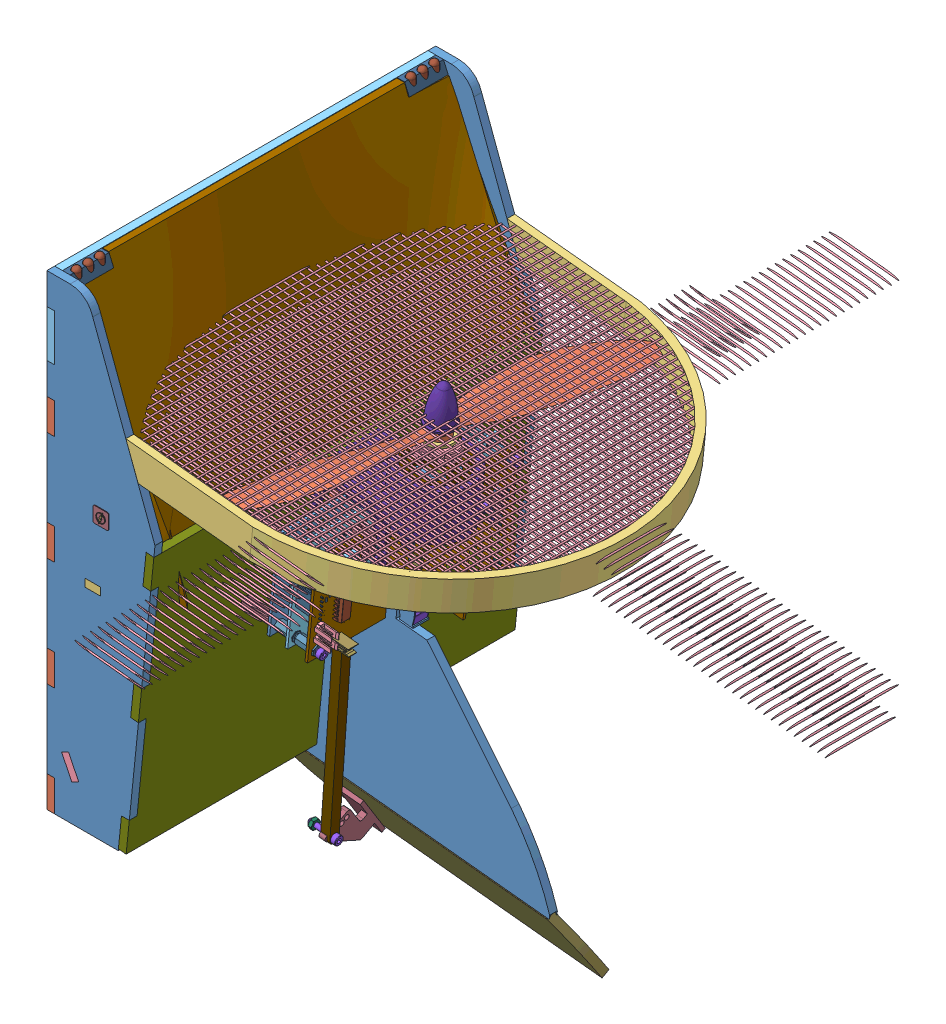
SolidWorks assembly AssTotaleSimu3, configuration Défaut. Lengths in mm. (continued)
Components (placement in the parent): (continued)
- AssStructSimu-1: AssStructSimu [Défaut] at (-125.7658 -1.8483 624.6548) x (1 0 0) z (0 0 -1) size (253.25 324.59 251.6) (continued)
  - AssCarte-1: AssCarte [Défaut] at (38.0121 147.1029 290.772) x (-0.101852 0.9948 0) z (0.9948 0.101852 0) size (66.52 130.57 98.72) (continued)
    - carte_onduleur_v3-1: carte_onduleur_v3 [Défaut] at (-131.8199 12.0892 20.7912) size (66.52 130.57 82.34) (continued)
      - RC2_2-1: RC2_2 [Défaut] at (-22 0.18 -0.803) x (-1 0 0) z (0 0 -1) size (2.34 1.04 0.5) (continued)
        - Open CASCADE STEP translator 6.8 1.12.1-1: Open CASCADE STEP translator 6.8 1.12.1 [Défaut] at origin size (2.34 1.04 0.5) (continued)
          - Pin_2_2-1: Pin_2_2 [Défaut] at origin size (0.51 1.02 0.5)
      - RC3_1-1: RC3_1 [Défaut] at (-20.9336 -14.5 -0.803) x (1 0 0) z (0 0 -1) size (2.34 1.04 0.5)
        - Open CASCADE STEP translator 6.8 1.12.1-1: Open CASCADE STEP translator 6.8 1.12.1 [Défaut] at origin size (2.34 1.04 0.5)
          - Body_1_3-1: Body_1_3 [Défaut] at origin size (2.29 1.04 0.43)
          - Pin_1_2-1: Pin_1_2 [Défaut] at (0.3048 0 0) x (-1 0 0) z (0 0 1) size (0.51 1.02 0.5)
          - Pin_2_2-1: Pin_2_2 [Défaut] at origin size (0.51 1.02 0.5)
      - RC3_2-1: RC3_2 [Défaut] at (-22.3 -14.5 -0.803) x (-1 0 0) z (0 0 -1) size (2.34 1.04 0.5)
        - Open CASCADE STEP translator 6.8 1.12.1-1: Open CASCADE STEP translator 6.8 1.12.1 [Défaut] at origin size (2.34 1.04 0.5)
          - Body_1_3-1: Body_1_3 [Défaut] at origin size (2.29 1.04 0.43)
          - Pin_1_2-1: Pin_1_2 [Défaut] at (0.3048 0 0) x (-1 0 0) z (0 0 1) size (0.51 1.02 0.5)
          - Pin_2_2-1: Pin_2_2 [Défaut] at origin size (0.51 1.02 0.5)
      - U_MES_CUR-1: U_MES_CUR [Défaut] at (-11.5 6.7816 0.803) size (2.54 2.41 0.76)
        - Open CASCADE STEP translator 6.8 1.32.1-1: Open CASCADE STEP translator 6.8 1.32.1 [Défaut] at origin size (2.54 2.41 0.76)
          - Body_1_5-1: Body_1_5 [Défaut] at origin size (2.54 1.27 0.71)
          - Pin_1_3-1: Pin_1_3 [Défaut] at (-2.1082 0.2286 0) x (0 -1 0) z (0 0 1) size (1.14 0.25 0.47)
          - Pin_2_3-1: Pin_2_3 [Défaut] at (-0.2032 2.1336 0) x (0 -1 0) z (0 0 1) size (1.14 0.25 0.47)
      - CARTE_ALIM-1: CARTE_ALIM [Défaut] at (-6.4 -57.2 0.803) size (60 130 18.35)
        - Open CASCADE STEP translator 6.8 1.33.1-1: Open CASCADE STEP translator 6.8 1.33.1 [Défaut] at origin size (60 130 18.35)
          - Body_1_6-1: Body_1_6 [Défaut] at (7 56 -12) size (60 130 18.35)
            - 1_3-1: 1_3 [Défaut] at origin size (60 130 1.61)
            - 13_3-1: 13_3 [Défaut] at (0.4717 -40.93 0.803) x (0 1 0) z (0 0 1) size (5.65 4.9 1.7)
              - =_[0_1_1_4]_3-1: =_[0_1_1_4]_3 [Défaut] at origin size (5.65 4.9 1.7)
                - 2-1: 2 [Défaut] at origin size (3.75 4.9 1.53)
                - 3-1: 3 [Défaut] at origin size (0.95 0.51 1.06)
                - 4-1: 4 [Défaut] at origin size (0.95 0.51 1.06)
                - 5_2-1: 5_2 [Défaut] at origin size (0.95 0.51 1.06)
                - 6-1: 6 [Défaut] at origin size (0.95 0.51 1.06)
                - 7-1: 7 [Défaut] at (10.8 -5.08 0) x (-1 0 0) z (0 0 1) size (0.95 0.51 1.06)
                - 8_2-1: 8_2 [Défaut] at (10.8 -2.54 0) x (-1 0 0) z (0 0 1) size (0.95 0.51 1.06)
                - 9-1: 9 [Défaut] at (10.8 0 0) x (-1 0 0) z (0 0 1) size (0.95 0.51 1.06)
                - 10-1: 10 [Défaut] at (10.8 2.54 0) x (-1 0 0) z (0 0 1) size (0.95 0.51 1.06)
                - 11_2-1: 11_2 [Défaut] at (5.4 -1.27 0) x (-1 0 0) z (0 0 1) size (4.25 2.34 1.06)
            - 18-1: 18 [Défaut] at (-2.5283 -37.23 0.803) x (0 -1 0) z (0 0 1) size (2.34 1.04 0.5)
              - =_[0_1_1_16]-1: =_[0_1_1_16] [Défaut] at origin size (2.34 1.04 0.5)
                - 14_2-1: 14_2 [Défaut] at origin size (2.29 1.04 0.43)
                - 15_2-1: 15_2 [Défaut] at (0.3048 0 0) x (-1 0 0) z (0 0 1) size (0.51 1.02 0.5)
                - 16_2-1: 16_2 [Défaut] at origin size (0.51 1.02 0.5)
            - 21_2-1: 21_2 [Défaut] at (-2.2263 -24.628 -0.803) x (1 0 0) z (0 0 -1) size (8.01 8 14.24)
              - =_[0_1_1_21]-1: =_[0_1_1_21] [Défaut] at origin size (8.01 8 14.24)
                - 19-1: 19 [Défaut] at (1.8 0 0) x (1 0 0) z (0 -1 0) size (8.01 14.24 8)
            - 23_2-1: 23_2 [Défaut] at (1.2381 -31.53 0.803) size (2.34 1.04 0.5)
              - =_[0_1_1_16]-1: =_[0_1_1_16] [Défaut] at origin size (2.34 1.04 0.5)
                - 14_2-1: 14_2 [Défaut] at origin size (2.29 1.04 0.43)
                - 15_2-1: 15_2 [Défaut] at (0.3048 0 0) x (-1 0 0) z (0 0 1) size (0.51 1.02 0.5)
                - 16_2-1: 16_2 [Défaut] at origin size (0.51 1.02 0.5)
            - 28-1: 28 [Défaut] at (5 29.8636 0.803) x (0 -1 0) z (0 0 1) size (3.35 1.3 0.55)
              - =_[0_1_1_25]_2-1: =_[0_1_1_25]_2 [Défaut] at origin size (3.35 1.3 0.55)
                - 24-1: 24 [Défaut] at origin size (3.3 1.3 0.48)
                - 25_2-1: 25_2 [Défaut] at (0.5588 0 0) x (-1 0 0) z (0 0 1) size (0.76 1.27 0.55)
                - 26_2-1: 26_2 [Défaut] at origin size (0.76 1.27 0.55)
            - 30-1: 30 [Défaut] at (6.7 29.8636 0.803) x (0 -1 0) z (0 0 1) size (2.34 1.04 0.5)
              - =_[0_1_1_16]-1: =_[0_1_1_16] [Défaut] at origin size (2.34 1.04 0.5)
                - 14_2-1: 14_2 [Défaut] at origin size (2.29 1.04 0.43)
                - 15_2-1: 15_2 [Défaut] at (0.3048 0 0) x (-1 0 0) z (0 0 1) size (0.51 1.02 0.5)
                - 16_2-1: 16_2 [Défaut] at origin size (0.51 1.02 0.5)
            - 35_2-1: 35_2 [Défaut] at (-2.5 -46.37 0.803) x (0 1 0) z (0 0 1) size (3.4 2.06 0.79)
              - =_[0_1_1_31]-1: =_[0_1_1_31] [Défaut] at origin size (3.4 2.06 0.79)
                - 31_2-1: 31_2 [Défaut] at origin size (3.3 2.06 0.69)
                - 32_3-1: 32_3 [Défaut] at (0.5588 0 0) x (-1 0 0) z (0 0 1) size (0.81 2.03 0.79)
                - 33_3-1: 33_3 [Défaut] at origin size (0.81 2.03 0.79)
            - 37-1: 37 [Défaut] at (5 31.43 0.803) x (0 1 0) z (0 0 1) size (2.34 1.04 0.5)
              - =_[0_1_1_16]-1: =_[0_1_1_16] [Défaut] at origin size (2.34 1.04 0.5)
                - 14_2-1: 14_2 [Défaut] at origin size (2.29 1.04 0.43)
                - 15_2-1: 15_2 [Défaut] at (0.3048 0 0) x (-1 0 0) z (0 0 1) size (0.51 1.02 0.5)
                - 16_2-1: 16_2 [Défaut] at origin size (0.51 1.02 0.5)
            - 39-1: 39 [Défaut] at (-0.2 35.63 0.803) x (-1 0 0) z (0 0 1) size (2.34 1.04 0.5)
              - =_[0_1_1_16]-1: =_[0_1_1_16] [Défaut] at origin size (2.34 1.04 0.5)
                - 14_2-1: 14_2 [Défaut] at origin size (2.29 1.04 0.43)
                - 15_2-1: 15_2 [Défaut] at (0.3048 0 0) x (-1 0 0) z (0 0 1) size (0.51 1.02 0.5)
                - 16_2-1: 16_2 [Défaut] at origin size (0.51 1.02 0.5)
            - 41-1: 41 [Défaut] at (2.9 -45.5036 0.803) x (0 1 0) z (0 0 1) size (2.34 1.04 0.5)
              - =_[0_1_1_16]-1: =_[0_1_1_16] [Défaut] at origin size (2.34 1.04 0.5)
                - 14_2-1: 14_2 [Défaut] at origin size (2.29 1.04 0.43)
                - 15_2-1: 15_2 [Défaut] at (0.3048 0 0) x (-1 0 0) z (0 0 1) size (0.51 1.02 0.5)
                - 16_2-1: 16_2 [Défaut] at origin size (0.51 1.02 0.5)
            - 43-1: 43 [Défaut] at (17.1348 -42.6272 0.803) x (0 1 0) z (0 0 1) size (2.34 1.04 0.5)
              - =_[0_1_1_16]-1: =_[0_1_1_16] [Défaut] at origin size (2.34 1.04 0.5)
                - 14_2-1: 14_2 [Défaut] at origin size (2.29 1.04 0.43)
                - 15_2-1: 15_2 [Défaut] at (0.3048 0 0) x (-1 0 0) z (0 0 1) size (0.51 1.02 0.5)
                - 16_2-1: 16_2 [Défaut] at origin size (0.51 1.02 0.5)
            - 48_2-1: 48_2 [Défaut] at (-5.4717 -39.01 0.803) x (-1 0 0) z (0 0 1) size (4.19 3.4 1.75)
              - =_[0_1_1_40]-1: =_[0_1_1_40] [Défaut] at origin size (4.19 3.4 1.75)
                - 44_2-1: 44_2 [Défaut] at origin size (3.75 3.38 1.73)
                - 45_2-1: 45_2 [Défaut] at (0.438 0 0) x (-1 0 0) z (0 0 1) size (0.53 3.4 1.75)
                - 46_2-1: 46_2 [Défaut] at origin size (0.52 3.4 1.75)
            - 53-1: 53 [Défaut] at (0.9 35.63 0.803) size (2.34 1.04 0.5)
              - =_[0_1_1_45]-1: =_[0_1_1_45] [Défaut] at origin size (2.34 1.04 0.5)
                - 49_3-1: 49_3 [Défaut] at origin size (2.29 1.04 0.43)
                - 50-1: 50 [Défaut] at (0.3048 0 0) x (-1 0 0) z (0 0 1) size (0.51 1.02 0.5)
                - 51-1: 51 [Défaut] at origin size (0.51 1.02 0.5)
            - 55_2-1: 55_2 [Défaut] at (1.3 -45.5036 0.803) x (0 1 0) z (0 0 1) size (2.34 1.04 0.5)
              - =_[0_1_1_45]-1: =_[0_1_1_45] [Défaut] at origin size (2.34 1.04 0.5)
                - 49_3-1: 49_3 [Défaut] at origin size (2.29 1.04 0.43)
                - 50-1: 50 [Défaut] at (0.3048 0 0) x (-1 0 0) z (0 0 1) size (0.51 1.02 0.5)
                - 51-1: 51 [Défaut] at origin size (0.51 1.02 0.5)
            - 57_3-1: 57_3 [Défaut] at (17.2348 -43.9936 0.803) x (0 -1 0) z (0 0 1) size (2.34 1.04 0.5)
              - =_[0_1_1_45]-1: =_[0_1_1_45] [Défaut] at origin size (2.34 1.04 0.5)
                - 49_3-1: 49_3 [Défaut] at origin size (2.29 1.04 0.43)
                - 50-1: 50 [Défaut] at (0.3048 0 0) x (-1 0 0) z (0 0 1) size (0.51 1.02 0.5)
                - 51-1: 51 [Défaut] at origin size (0.51 1.02 0.5)
            - 65-1: 65 [Défaut] at (-4.8 30.93 0.803) x (-1 0 0) z (0 0 1) size (14.64 9.83 4.25)
              - =_[0_1_1_52]-1: =_[0_1_1_52] [Défaut] at origin size (14.64 9.83 4.25)
                - 63_2-1: 63_2 [Défaut] at (3 0 0) x (0 -1 0) z (0 0 1) size (9.83 14.64 4.25)
                  - =_[0_1_1_3]_5-1: =_[0_1_1_3]_5 [Défaut] at origin size (9.83 9.05 4.21)
                  - =_[0_1_1_4]_5-1: =_[0_1_1_4]_5 [Défaut] at origin size (9.48 7.76 1.21)
                  - =_[0_1_1_5]_5-1: =_[0_1_1_5]_5 [Défaut] at origin size (1.36 6.01 3.08)
                  - =_[0_1_1_6]_3-1: =_[0_1_1_6]_3 [Défaut] at origin size (1.36 6.01 3.08)
                  - =_[0_1_1_7]_3-1: =_[0_1_1_7]_3 [Défaut] at origin size (1.06 6.01 3.08)
            - 67-1: 67 [Défaut] at (13.5933 -37.5272 0.803) x (-1 0 0) z (0 0 1) size (2.34 1.04 0.5)
              - =_[0_1_1_16]-1: =_[0_1_1_16] [Défaut] at origin size (2.34 1.04 0.5)
                - 14_2-1: 14_2 [Défaut] at origin size (2.29 1.04 0.43)
                - 15_2-1: 15_2 [Défaut] at (0.3048 0 0) x (-1 0 0) z (0 0 1) size (0.51 1.02 0.5)
                - 16_2-1: 16_2 [Défaut] at origin size (0.51 1.02 0.5)
            - 70_2-1: 70_2 [Défaut] at (18.2733 -29.7272 0.803) x (0 1 0) z (0 0 1) size (6.06 4.95 1.88)
              - =_[0_1_1_61]-1: =_[0_1_1_61] [Défaut] at origin size (6.06 4.95 1.88)
                - 68-1: 68 [Défaut] x (1 0 0) z (0 -1 0) size (6.06 1.88 4.95)
            - 83-1: 83 [Défaut] at (-21.2 -38.07 0.803) x (-1 0 0) z (0 0 1) size (2.7 5.2 1.11)
              - =_[0_1_1_64]-1: =_[0_1_1_64] [Défaut] at origin size (2.7 5.2 1.11)
                - 84_2-1: 84_2 [Défaut] at (1.2 -4 0) x (0 1 0) z (0 0 1) size (5.2 2.7 1.11)
                  - =_[0_1_1_3]_6-1: =_[0_1_1_3]_6 [Défaut] at origin size (0.39 0.64 0.01)
                  - =_[0_1_1_4]_6-1: =_[0_1_1_4]_6 [Défaut] at origin size (0.6 1.9 0.2)
                  - =_[0_1_1_5]_6-1: =_[0_1_1_5]_6 [Défaut] at origin size (0.21 0.08 0.01)
                  - =_[0_1_1_6]_4-1: =_[0_1_1_6]_4 [Défaut] at origin size (0.6 1.9 0.2)
                  - =_[0_1_1_7]_4-1: =_[0_1_1_7]_4 [Défaut] at origin size (0.46 0.68 0.01)
                  - =_[0_1_1_8]_3-1: =_[0_1_1_8]_3 [Défaut] at origin size (0.38 0.66 0.01)
                  - =_[0_1_1_9]_2-1: =_[0_1_1_9]_2 [Défaut] at origin size (0.2 0.62 0.01)
                  - =_[0_1_1_10]_2-1: =_[0_1_1_10]_2 [Défaut] at origin size (4 2.7 1.1)
                  - =_[0_1_1_11]_2-1: =_[0_1_1_11]_2 [Défaut] at origin size (0.46 0.63 0.01)
                  - =_[0_1_1_12]_2-1: =_[0_1_1_12]_2 [Défaut] at origin size (0.56 0.68 0.01)
            - 86_2-1: 86_2 [Défaut] at (12.8933 -35.4272 0.803) x (0 1 0) z (0 0 1) size (2.7 5.2 1.11)
              - =_[0_1_1_77]-1: =_[0_1_1_77] [Défaut] at origin size (2.7 5.2 1.11)
                - 84_2-1: 84_2 [Défaut] at (1.2 -4 0) x (0 1 0) z (0 0 1) size (5.2 2.7 1.11)
                  - =_[0_1_1_3]_6-1: =_[0_1_1_3]_6 [Défaut] at origin size (0.39 0.64 0.01)
                  - =_[0_1_1_4]_6-1: =_[0_1_1_4]_6 [Défaut] at origin size (0.6 1.9 0.2)
                  - =_[0_1_1_5]_6-1: =_[0_1_1_5]_6 [Défaut] at origin size (0.21 0.08 0.01)
                  - =_[0_1_1_6]_4-1: =_[0_1_1_6]_4 [Défaut] at origin size (0.6 1.9 0.2)
                  - =_[0_1_1_7]_4-1: =_[0_1_1_7]_4 [Défaut] at origin size (0.46 0.68 0.01)
                  - =_[0_1_1_8]_3-1: =_[0_1_1_8]_3 [Défaut] at origin size (0.38 0.66 0.01)
                  - =_[0_1_1_9]_2-1: =_[0_1_1_9]_2 [Défaut] at origin size (0.2 0.62 0.01)
                  - =_[0_1_1_10]_2-1: =_[0_1_1_10]_2 [Défaut] at origin size (4 2.7 1.1)
                  - =_[0_1_1_11]_2-1: =_[0_1_1_11]_2 [Défaut] at origin size (0.46 0.63 0.01)
                  - =_[0_1_1_12]_2-1: =_[0_1_1_12]_2 [Défaut] at origin size (0.56 0.68 0.01)
            - 92_2-1: 92_2 [Défaut] at (20.9933 -39.3272 0.803) x (0 -1 0) z (0 0 1) size (2.79 1.98 0.64)
              - =_[0_1_1_79]-1: =_[0_1_1_79] [Défaut] at origin size (2.79 1.98 0.64)
                - 87-1: 87 [Défaut] at origin size (2.79 1.02 0.58)
                - 88-1: 88 [Défaut] x (0 -1 0) z (0 0 1) size (0.42 0.38 0.38)
                - 89-1: 89 [Défaut] at (-2.8448 -0.9652 0) x (0 1 0) z (0 0 1) size (0.55 0.38 0.38)
                - 90-1: 90 [Défaut] at (-0.9652 -2.8448 0) x (0 1 0) z (0 0 1) size (0.55 0.38 0.38)
            - 98-1: 98 [Défaut] at (-17.7 -48.47 0.803) x (0 -1 0) z (0 0 1) size (2.54 1.98 0.64)
              - =_[0_1_1_85]-1: =_[0_1_1_85] [Défaut] at origin size (2.54 1.98 0.64)
                - 93-1: 93 [Défaut] at origin size (2.54 1.14 0.58)
                - 94-1: 94 [Défaut] x (0 -1 0) z (0 0 1) size (0.43 0.51 0.38)
                - 95-1: 95 [Défaut] at (1.8796 1.8796 0) x (0 -1 0) z (0 0 1) size (0.43 0.51 0.38)
                - 96-1: 96 [Défaut] at (-0.9652 -2.8448 0) x (0 1 0) z (0 0 1) size (0.41 0.51 0.38)
            - 100-1: 100 [Défaut] at (24.3933 -43.2272 0.803) size (2.79 1.98 0.64)
              - =_[0_1_1_79]-1: =_[0_1_1_79] [Défaut] at origin size (2.79 1.98 0.64)
                - 87-1: 87 [Défaut] at origin size (2.79 1.02 0.58)
                - 88-1: 88 [Défaut] x (0 -1 0) z (0 0 1) size (0.42 0.38 0.38)
                - 89-1: 89 [Défaut] at (-2.8448 -0.9652 0) x (0 1 0) z (0 0 1) size (0.55 0.38 0.38)
                - 90-1: 90 [Défaut] at (-0.9652 -2.8448 0) x (0 1 0) z (0 0 1) size (0.55 0.38 0.38)
            - 102-1: 102 [Défaut] at (21.4933 -44.4272 0.803) x (0 -1 0) z (0 0 1) size (2.79 1.98 0.64)
              - =_[0_1_1_79]-1: =_[0_1_1_79] [Défaut] at origin size (2.79 1.98 0.64)
                - 87-1: 87 [Défaut] at origin size (2.79 1.02 0.58)
                - 88-1: 88 [Défaut] x (0 -1 0) z (0 0 1) size (0.42 0.38 0.38)
                - 89-1: 89 [Défaut] at (-2.8448 -0.9652 0) x (0 1 0) z (0 0 1) size (0.55 0.38 0.38)
                - 90-1: 90 [Défaut] at (-0.9652 -2.8448 0) x (0 1 0) z (0 0 1) size (0.55 0.38 0.38)
            - 107-1: 107 [Défaut] at (23.1933 -29.1272 -0.803) x (0 1 0) z (0 0 -1) size (9.6 14.35 5)
              - =_[0_1_1_93]-1: =_[0_1_1_93] [Défaut] at origin size (9.6 14.35 5)
                - 105-1: 105 [Défaut] at (0.5 -1 2) x (-1 0 0) z (0 0 1) size (9.6 14.35 5)
                  - =_[0_1_1_3]_7-1: =_[0_1_1_3]_7 [Défaut] at origin size (9.6 12.75 5)
                  - =_[0_1_1_4]_7-1: =_[0_1_1_4]_7 [Défaut] at origin size (2.2 1.6 2.2)
            - 109-1: 109 [Défaut] at (25.4933 -41.1272 0.803) x (-1 0 0) z (0 0 1) size (2.34 1.04 0.5)
              - =_[0_1_1_45]-1: =_[0_1_1_45] [Défaut] at origin size (2.34 1.04 0.5)
                - 49_3-1: 49_3 [Défaut] at origin size (2.29 1.04 0.43)
                - 50-1: 50 [Défaut] at (0.3048 0 0) x (-1 0 0) z (0 0 1) size (0.51 1.02 0.5)
                - 51-1: 51 [Défaut] at origin size (0.51 1.02 0.5)
            - 111-1: 111 [Défaut] at (22.0269 -41.8272 0.803) x (-1 0 0) z (0 0 1) size (2.34 1.04 0.5)
              - =_[0_1_1_45]-1: =_[0_1_1_45] [Défaut] at origin size (2.34 1.04 0.5)
                - 49_3-1: 49_3 [Défaut] at origin size (2.29 1.04 0.43)
                - 50-1: 50 [Défaut] at (0.3048 0 0) x (-1 0 0) z (0 0 1) size (0.51 1.02 0.5)
                - 51-1: 51 [Défaut] at origin size (0.51 1.02 0.5)
            - 113-1: 113 [Défaut] at (-24.8 -36.7036 0.803) x (0 1 0) z (0 0 1) size (2.34 1.04 0.5)
              - =_[0_1_1_45]-1: =_[0_1_1_45] [Défaut] at origin size (2.34 1.04 0.5)
                - 49_3-1: 49_3 [Défaut] at origin size (2.29 1.04 0.43)
                - 50-1: 50 [Défaut] at (0.3048 0 0) x (-1 0 0) z (0 0 1) size (0.51 1.02 0.5)
                - 51-1: 51 [Défaut] at origin size (0.51 1.02 0.5)
            - 115-1: 115 [Défaut] at (-24.8 -40.3036 0.803) x (0 1 0) z (0 0 1) size (2.34 1.04 0.5)
              - =_[0_1_1_45]-1: =_[0_1_1_45] [Défaut] at origin size (2.34 1.04 0.5)
                - 49_3-1: 49_3 [Défaut] at origin size (2.29 1.04 0.43)
                - 50-1: 50 [Défaut] at (0.3048 0 0) x (-1 0 0) z (0 0 1) size (0.51 1.02 0.5)
                - 51-1: 51 [Défaut] at origin size (0.51 1.02 0.5)
            - 117-1: 117 [Défaut] at (-16 -48.27 0.803) x (0 -1 0) z (0 0 1) size (2.34 1.04 0.5)
              - =_[0_1_1_45]-1: =_[0_1_1_45] [Défaut] at origin size (2.34 1.04 0.5)
                - 49_3-1: 49_3 [Défaut] at origin size (2.29 1.04 0.43)
                - 50-1: 50 [Défaut] at (0.3048 0 0) x (-1 0 0) z (0 0 1) size (0.51 1.02 0.5)
                - 51-1: 51 [Défaut] at origin size (0.51 1.02 0.5)
            - 119-1: 119 [Défaut] at (-22.5189 -47.87 0.803) x (-1 0 0) z (0 0 1) size (2.34 1.04 0.5)
              - =_[0_1_1_45]-1: =_[0_1_1_45] [Défaut] at origin size (2.34 1.04 0.5)
                - 49_3-1: 49_3 [Défaut] at origin size (2.29 1.04 0.43)
                - 50-1: 50 [Défaut] at (0.3048 0 0) x (-1 0 0) z (0 0 1) size (0.51 1.02 0.5)
                - 51-1: 51 [Défaut] at origin size (0.51 1.02 0.5)
            - 121-1: 121 [Défaut] at (22.3933 -38.9272 0.803) size (2.34 1.04 0.5)
              - =_[0_1_1_45]-1: =_[0_1_1_45] [Défaut] at origin size (2.34 1.04 0.5)
                - 49_3-1: 49_3 [Défaut] at origin size (2.29 1.04 0.43)
                - 50-1: 50 [Défaut] at (0.3048 0 0) x (-1 0 0) z (0 0 1) size (0.51 1.02 0.5)
                - 51-1: 51 [Défaut] at origin size (0.51 1.02 0.5)
            - 123-1: 123 [Défaut] at (22.0933 -36.4272 0.803) x (-1 0 0) z (0 0 1) size (2.34 1.04 0.5)
              - =_[0_1_1_45]-1: =_[0_1_1_45] [Défaut] at origin size (2.34 1.04 0.5)
                - 49_3-1: 49_3 [Défaut] at origin size (2.29 1.04 0.43)
                - 50-1: 50 [Défaut] at (0.3048 0 0) x (-1 0 0) z (0 0 1) size (0.51 1.02 0.5)
                - 51-1: 51 [Défaut] at origin size (0.51 1.02 0.5)
            - 125-1: 125 [Défaut] at (22.3933 -32.0272 0.803) x (0 -1 0) z (0 0 1) size (2.34 1.04 0.5)
              - =_[0_1_1_45]-1: =_[0_1_1_45] [Défaut] at origin size (2.34 1.04 0.5)
                - 49_3-1: 49_3 [Défaut] at origin size (2.29 1.04 0.43)
                - 50-1: 50 [Défaut] at (0.3048 0 0) x (-1 0 0) z (0 0 1) size (0.51 1.02 0.5)
                - 51-1: 51 [Défaut] at origin size (0.51 1.02 0.5)
            - 127-1: 127 [Défaut] at (17.9597 -23.1272 0.803) size (2.34 1.04 0.5)
              - =_[0_1_1_16]-1: =_[0_1_1_16] [Défaut] at origin size (2.34 1.04 0.5)
                - 14_2-1: 14_2 [Défaut] at origin size (2.29 1.04 0.43)
                - 15_2-1: 15_2 [Défaut] at (0.3048 0 0) x (-1 0 0) z (0 0 1) size (0.51 1.02 0.5)
                - 16_2-1: 16_2 [Défaut] at origin size (0.51 1.02 0.5)
            - 129-1: 129 [Défaut] at (20.0269 -24.9272 0.803) x (-1 0 0) z (0 0 1) size (2.34 1.04 0.5)
              - =_[0_1_1_16]-1: =_[0_1_1_16] [Défaut] at origin size (2.34 1.04 0.5)
                - 14_2-1: 14_2 [Défaut] at origin size (2.29 1.04 0.43)
                - 15_2-1: 15_2 [Défaut] at (0.3048 0 0) x (-1 0 0) z (0 0 1) size (0.51 1.02 0.5)
                - 16_2-1: 16_2 [Défaut] at origin size (0.51 1.02 0.5)
            - 131-1: 131 [Défaut] at (16.9933 -37.5272 0.803) x (-1 0 0) z (0 0 1) size (2.34 1.04 0.5)
              - =_[0_1_1_45]-1: =_[0_1_1_45] [Défaut] at origin size (2.34 1.04 0.5)
                - 49_3-1: 49_3 [Défaut] at origin size (2.29 1.04 0.43)
                - 50-1: 50 [Défaut] at (0.3048 0 0) x (-1 0 0) z (0 0 1) size (0.51 1.02 0.5)
                - 51-1: 51 [Défaut] at origin size (0.51 1.02 0.5)
            - 136-1: 136 [Défaut] at (3.2957 -29.23 0.803) x (-1 0 0) z (0 0 1) size (4.78 2.79 2.03)
              - =_[0_1_1_110]_2-1: =_[0_1_1_110]_2 [Défaut] at origin size (4.78 2.79 2.03)
                - 132-1: 132 [Défaut] at origin size (4.32 2.79 1.78)
                - 133-1: 133 [Défaut] at (0.4572 0 0) x (-1 0 0) z (0 0 1) size (1.02 1.27 1.32)
                - 134-1: 134 [Défaut] at origin size (1.02 1.27 1.32)
            - 141-1: 141 [Défaut] at (0.2436 -33.3673 0.803) size (3.35 1.3 0.55)
              - =_[0_1_1_115]_2-1: =_[0_1_1_115]_2 [Défaut] at origin size (3.35 1.3 0.55)
                - 137-1: 137 [Défaut] at origin size (3.3 1.3 0.48)
                - 138-1: 138 [Défaut] at (0.5588 0 0) x (-1 0 0) z (0 0 1) size (0.76 1.27 0.55)
                - 139-1: 139 [Défaut] at origin size (0.76 1.27 0.55)
            - 143_2-1: 143_2 [Défaut] at (-0.3 -45.47 0.803) x (0 1 0) z (0 0 1) size (2.34 1.04 0.5)
              - =_[0_1_1_16]-1: =_[0_1_1_16] [Défaut] at origin size (2.34 1.04 0.5)
                - 14_2-1: 14_2 [Défaut] at origin size (2.29 1.04 0.43)
                - 15_2-1: 15_2 [Défaut] at (0.3048 0 0) x (-1 0 0) z (0 0 1) size (0.51 1.02 0.5)
                - 16_2-1: 16_2 [Défaut] at origin size (0.51 1.02 0.5)
            - 145-1: 145 [Défaut] at (6.6 31.13 0.803) x (0 1 0) z (0 0 1) size (3.35 1.3 0.55)
              - =_[0_1_1_25]_2-1: =_[0_1_1_25]_2 [Défaut] at origin size (3.35 1.3 0.55)
                - 24-1: 24 [Défaut] at origin size (3.3 1.3 0.48)
                - 25_2-1: 25_2 [Défaut] at (0.5588 0 0) x (-1 0 0) z (0 0 1) size (0.76 1.27 0.55)
                - 26_2-1: 26_2 [Défaut] at origin size (0.76 1.27 0.55)
            - 148-1: 148 [Défaut] at (-7.5 -56.57 0.803) size (15.24 2.54 7.37)
              - =_[0_1_1_122]_2-1: =_[0_1_1_122]_2 [Défaut] at origin size (15.24 2.54 7.37)
                - 146-1: 146 [Défaut] at (6.3 0 1) x (1 0 0) z (0 -1 0) size (15.24 7.37 2.54)
      - COMP1-1: COMP1 [Défaut] at (-16.3 -36.2 0.803) x (-1 0 0) z (0 0 1) size (2.03 1.88 0.51)
        - Open CASCADE STEP translator 6.8 1.34.1-1: Open CASCADE STEP translator 6.8 1.34.1 [Défaut] at origin size (2.03 1.88 0.51)
          - Body_1_6-1: Body_1_6 [Défaut] at origin size (2.03 1.02 0.46)
          - Pin_1_4-1: Pin_1_4 [Défaut] x (0 1 0) z (0 0 1) size (0.45 0.25 0.32)
          - Pin_2_4-1: Pin_2_4 [Défaut] at (0.65 -0.65 0) x (0 1 0) z (0 0 1) size (0.45 0.25 0.32)
          - Pin_3-1: Pin_3 [Défaut] at (1.3 -1.3 0) x (0 1 0) z (0 0 1) size (0.45 0.25 0.32)
          - Pin_4-1: Pin_4 [Défaut] at (-0.5 3.1 0) x (0 -1 0) z (0 0 1) size (0.41 0.25 0.32)
          - Pin_5-1: Pin_5 [Défaut] at (-1.8 1.8 0) x (0 -1 0) z (0 0 1) size (0.41 0.25 0.32)
      - COMP2-1: COMP2 [Défaut] at (-14.3 -9.6 0.803) x (-1 0 0) z (0 0 1) size (2.03 1.88 0.51)
        - Open CASCADE STEP translator 6.8 1.34.1-1: Open CASCADE STEP translator 6.8 1.34.1 [Défaut] at origin size (2.03 1.88 0.51)
          - Body_1_6-1: Body_1_6 [Défaut] at origin size (2.03 1.02 0.46)
          - Pin_1_4-1: Pin_1_4 [Défaut] x (0 1 0) z (0 0 1) size (0.45 0.25 0.32)
          - Pin_2_4-1: Pin_2_4 [Défaut] at (0.65 -0.65 0) x (0 1 0) z (0 0 1) size (0.45 0.25 0.32)
          - Pin_3-1: Pin_3 [Défaut] at (1.3 -1.3 0) x (0 1 0) z (0 0 1) size (0.45 0.25 0.32)
          - Pin_4-1: Pin_4 [Défaut] at (-0.5 3.1 0) x (0 -1 0) z (0 0 1) size (0.41 0.25 0.32)
          - Pin_5-1: Pin_5 [Défaut] at (-1.8 1.8 0) x (0 -1 0) z (0 0 1) size (0.41 0.25 0.32)
      - COMP3-1: COMP3 [Défaut] at (-15.9 -23.2 0.803) x (-1 0 0) z (0 0 1) size (2.03 1.88 0.51)
        - Open CASCADE STEP translator 6.8 1.34.1-1: Open CASCADE STEP translator 6.8 1.34.1 [Défaut] at origin size (2.03 1.88 0.51)
          - Body_1_6-1: Body_1_6 [Défaut] at origin size (2.03 1.02 0.46)
          - Pin_1_4-1: Pin_1_4 [Défaut] x (0 1 0) z (0 0 1) size (0.45 0.25 0.32)
          - Pin_2_4-1: Pin_2_4 [Défaut] at (0.65 -0.65 0) x (0 1 0) z (0 0 1) size (0.45 0.25 0.32)
          - Pin_3-1: Pin_3 [Défaut] at (1.3 -1.3 0) x (0 1 0) z (0 0 1) size (0.45 0.25 0.32)
          - Pin_4-1: Pin_4 [Défaut] at (-0.5 3.1 0) x (0 -1 0) z (0 0 1) size (0.41 0.25 0.32)
          - Pin_5-1: Pin_5 [Défaut] at (-1.8 1.8 0) x (0 -1 0) z (0 0 1) size (0.41 0.25 0.32)
      - CP1-1: CP1 [Défaut] at (-18.9 -38.2 0.803) x (0 1 0) z (0 0 1) size (2.34 1.04 0.5)
        - Open CASCADE STEP translator 6.8 1.6.1-1: Open CASCADE STEP translator 6.8 1.6.1 [Défaut] at origin size (2.34 1.04 0.5)
          - Body_1-1: Body_1 [Défaut] at origin size (2.29 1.04 0.43)
          - Pin_1-1: Pin_1 [Défaut] at (0.3048 0 0) x (-1 0 0) z (0 0 1) size (0.51 1.02 0.5)
          - Pin_2-1: Pin_2 [Défaut] at origin size (0.51 1.02 0.5)
      - CP2-1: CP2 [Défaut] at (-16.9 -11.6 0.803) x (0 1 0) z (0 0 1) size (2.34 1.04 0.5)
        - Open CASCADE STEP translator 6.8 1.6.1-1: Open CASCADE STEP translator 6.8 1.6.1 [Défaut] at origin size (2.34 1.04 0.5)
          - Body_1-1: Body_1 [Défaut] at origin size (2.29 1.04 0.43)
          - Pin_1-1: Pin_1 [Défaut] at (0.3048 0 0) x (-1 0 0) z (0 0 1) size (0.51 1.02 0.5)
          - Pin_2-1: Pin_2 [Défaut] at origin size (0.51 1.02 0.5)
      - CP3-1: CP3 [Défaut] at (-18.5 -25.2 0.803) x (0 1 0) z (0 0 1) size (2.34 1.04 0.5)
        - Open CASCADE STEP translator 6.8 1.6.1-1: Open CASCADE STEP translator 6.8 1.6.1 [Défaut] at origin size (2.34 1.04 0.5)
          - Body_1-1: Body_1 [Défaut] at origin size (2.29 1.04 0.43)
          - Pin_1-1: Pin_1 [Défaut] at (0.3048 0 0) x (-1 0 0) z (0 0 1) size (0.51 1.02 0.5)
          - Pin_2-1: Pin_2 [Défaut] at origin size (0.51 1.02 0.5)
      - C_DEC_COM1-1: C_DEC_COM1 [Défaut] at (-15 -36 0.803) x (0 -1 0) z (0 0 1) size (2.34 1.04 0.5)
        - Open CASCADE STEP translator 6.8 1.6.1-1: Open CASCADE STEP translator 6.8 1.6.1 [Défaut] at origin size (2.34 1.04 0.5)
          - Body_1-1: Body_1 [Défaut] at origin size (2.29 1.04 0.43)
          - Pin_1-1: Pin_1 [Défaut] at (0.3048 0 0) x (-1 0 0) z (0 0 1) size (0.51 1.02 0.5)
          - Pin_2-1: Pin_2 [Défaut] at origin size (0.51 1.02 0.5)
      - C_DEC_COMP2-1: C_DEC_COMP2 [Défaut] at (-13 -9.3 0.803) x (0 -1 0) z (0 0 1) size (2.34 1.04 0.5)
        - Open CASCADE STEP translator 6.8 1.6.1-1: Open CASCADE STEP translator 6.8 1.6.1 [Défaut] at origin size (2.34 1.04 0.5)
          - Body_1-1: Body_1 [Défaut] at origin size (2.29 1.04 0.43)
          - Pin_1-1: Pin_1 [Défaut] at (0.3048 0 0) x (-1 0 0) z (0 0 1) size (0.51 1.02 0.5)
          - Pin_2-1: Pin_2 [Défaut] at origin size (0.51 1.02 0.5)
      - C_DEC_COMP3-1: C_DEC_COMP3 [Défaut] at (-14.6 -22.9 0.803) x (0 -1 0) z (0 0 1) size (2.34 1.04 0.5)
        - Open CASCADE STEP translator 6.8 1.6.1-1: Open CASCADE STEP translator 6.8 1.6.1 [Défaut] at origin size (2.34 1.04 0.5)
          - Body_1-1: Body_1 [Défaut] at origin size (2.29 1.04 0.43)
          - Pin_1-1: Pin_1 [Défaut] at (0.3048 0 0) x (-1 0 0) z (0 0 1) size (0.51 1.02 0.5)
          - Pin_2-1: Pin_2 [Défaut] at origin size (0.51 1.02 0.5)
      - D_VBAT-1: D_VBAT [Défaut] at (-1.2 46.4 0.803) x (0 -1 0) z (0 0 1) size (2.34 1.04 0.5)
        - Open CASCADE STEP translator 6.8 1.6.1-1: Open CASCADE STEP translator 6.8 1.6.1 [Défaut] at origin size (2.34 1.04 0.5)
          - Body_1-1: Body_1 [Défaut] at origin size (2.29 1.04 0.43)
          - Pin_1-1: Pin_1 [Défaut] at (0.3048 0 0) x (-1 0 0) z (0 0 1) size (0.51 1.02 0.5)
          - Pin_2-1: Pin_2 [Défaut] at origin size (0.51 1.02 0.5)
      - D_3V-1: D_3V [Défaut] at (1.3 46.3 0.803) x (0 -1 0) z (0 0 1) size (2.34 1.04 0.5)
        - Open CASCADE STEP translator 6.8 1.6.1-1: Open CASCADE STEP translator 6.8 1.6.1 [Défaut] at origin size (2.34 1.04 0.5)
          - Body_1-1: Body_1 [Défaut] at origin size (2.29 1.04 0.43)
          - Pin_1-1: Pin_1 [Défaut] at (0.3048 0 0) x (-1 0 0) z (0 0 1) size (0.51 1.02 0.5)
          - Pin_2-1: Pin_2 [Défaut] at origin size (0.51 1.02 0.5)
      - D_5V-1: D_5V [Défaut] at (-3.7 46.4 0.803) x (0 -1 0) z (0 0 1) size (2.34 1.04 0.5)
        - Open CASCADE STEP translator 6.8 1.6.1-1: Open CASCADE STEP translator 6.8 1.6.1 [Défaut] at origin size (2.34 1.04 0.5)
          - Body_1-1: Body_1 [Défaut] at origin size (2.29 1.04 0.43)
          - Pin_1-1: Pin_1 [Défaut] at (0.3048 0 0) x (-1 0 0) z (0 0 1) size (0.51 1.02 0.5)
          - Pin_2-1: Pin_2 [Défaut] at origin size (0.51 1.02 0.5)
      - R1_1-1: R1_1 [Défaut] at (-20.2 -36.1 0.803) x (-1 0 0) z (0 0 1) size (2.34 1.04 0.5)
        - Open CASCADE STEP translator 6.8 1.12.1-1: Open CASCADE STEP translator 6.8 1.12.1 [Défaut] at origin size (2.34 1.04 0.5)
          - Body_1_3-1: Body_1_3 [Défaut] at origin size (2.29 1.04 0.43)
          - Pin_1_2-1: Pin_1_2 [Défaut] at (0.3048 0 0) x (-1 0 0) z (0 0 1) size (0.51 1.02 0.5)
          - Pin_2_2-1: Pin_2_2 [Défaut] at origin size (0.51 1.02 0.5)
      - R1_2-1: R1_2 [Défaut] at (-15.5 -34.6 0.803) x (-1 0 0) z (0 0 1) size (2.34 1.04 0.5)
        - Open CASCADE STEP translator 6.8 1.12.1-1: Open CASCADE STEP translator 6.8 1.12.1 [Défaut] at origin size (2.34 1.04 0.5)
          - Body_1_3-1: Body_1_3 [Défaut] at origin size (2.29 1.04 0.43)
          - Pin_1_2-1: Pin_1_2 [Défaut] at (0.3048 0 0) x (-1 0 0) z (0 0 1) size (0.51 1.02 0.5)
          - Pin_2_2-1: Pin_2_2 [Défaut] at origin size (0.51 1.02 0.5)
      - R1_3-1: R1_3 [Défaut] at (-20.3 -39.9 0.803) x (-1 0 0) z (0 0 1) size (2.34 1.04 0.5)
        - Open CASCADE STEP translator 6.8 1.12.1-1: Open CASCADE STEP translator 6.8 1.12.1 [Défaut] at origin size (2.34 1.04 0.5)
          - Body_1_3-1: Body_1_3 [Défaut] at origin size (2.29 1.04 0.43)
          - Pin_1_2-1: Pin_1_2 [Défaut] at (0.3048 0 0) x (-1 0 0) z (0 0 1) size (0.51 1.02 0.5)
          - Pin_2_2-1: Pin_2_2 [Défaut] at origin size (0.51 1.02 0.5)
      - R1_4-1: R1_4 [Défaut] at (-20.3 -38.1 0.803) x (-1 0 0) z (0 0 1) size (2.34 1.04 0.5)
        - Open CASCADE STEP translator 6.8 1.12.1-1: Open CASCADE STEP translator 6.8 1.12.1 [Défaut] at origin size (2.34 1.04 0.5)
          - Body_1_3-1: Body_1_3 [Défaut] at origin size (2.29 1.04 0.43)
          - Pin_1_2-1: Pin_1_2 [Défaut] at (0.3048 0 0) x (-1 0 0) z (0 0 1) size (0.51 1.02 0.5)
          - Pin_2_2-1: Pin_2_2 [Défaut] at origin size (0.51 1.02 0.5)
      - R1_5-1: R1_5 [Défaut] at (-17.1336 -39.7 0.803) size (2.34 1.04 0.5)
        - Open CASCADE STEP translator 6.8 1.12.1-1: Open CASCADE STEP translator 6.8 1.12.1 [Défaut] at origin size (2.34 1.04 0.5)
          - Body_1_3-1: Body_1_3 [Défaut] at origin size (2.29 1.04 0.43)
          - Pin_1_2-1: Pin_1_2 [Défaut] at (0.3048 0 0) x (-1 0 0) z (0 0 1) size (0.51 1.02 0.5)
          - Pin_2_2-1: Pin_2_2 [Défaut] at origin size (0.51 1.02 0.5)
      - R2_1-1: R2_1 [Défaut] at (-18.5 -9.5 0.803) x (-1 0 0) z (0 0 1) size (2.34 1.04 0.5)
        - Open CASCADE STEP translator 6.8 1.12.1-1: Open CASCADE STEP translator 6.8 1.12.1 [Défaut] at origin size (2.34 1.04 0.5)
          - Body_1_3-1: Body_1_3 [Défaut] at origin size (2.29 1.04 0.43)
          - Pin_1_2-1: Pin_1_2 [Défaut] at (0.3048 0 0) x (-1 0 0) z (0 0 1) size (0.51 1.02 0.5)
          - Pin_2_2-1: Pin_2_2 [Défaut] at origin size (0.51 1.02 0.5)
      - R2_2-1: R2_2 [Défaut] at (-13.1 -8 0.803) x (-1 0 0) z (0 0 1) size (2.34 1.04 0.5)
        - Open CASCADE STEP translator 6.8 1.12.1-1: Open CASCADE STEP translator 6.8 1.12.1 [Défaut] at origin size (2.34 1.04 0.5)
          - Body_1_3-1: Body_1_3 [Défaut] at origin size (2.29 1.04 0.43)
          - Pin_1_2-1: Pin_1_2 [Défaut] at (0.3048 0 0) x (-1 0 0) z (0 0 1) size (0.51 1.02 0.5)
          - Pin_2_2-1: Pin_2_2 [Défaut] at origin size (0.51 1.02 0.5)
      - R2_3-1: R2_3 [Défaut] at (-18.5 -11.2 0.803) x (-1 0 0) z (0 0 1) size (2.34 1.04 0.5)
        - Open CASCADE STEP translator 6.8 1.12.1-1: Open CASCADE STEP translator 6.8 1.12.1 [Défaut] at origin size (2.34 1.04 0.5)
          - Body_1_3-1: Body_1_3 [Défaut] at origin size (2.29 1.04 0.43)
          - Pin_1_2-1: Pin_1_2 [Défaut] at (0.3048 0 0) x (-1 0 0) z (0 0 1) size (0.51 1.02 0.5)
          - Pin_2_2-1: Pin_2_2 [Défaut] at origin size (0.51 1.02 0.5)
      - R2_4-1: R2_4 [Défaut] at (-18.5 -12.8 0.803) x (-1 0 0) z (0 0 1) size (2.34 1.04 0.5)
        - Open CASCADE STEP translator 6.8 1.12.1-1: Open CASCADE STEP translator 6.8 1.12.1 [Défaut] at origin size (2.34 1.04 0.5)
          - Body_1_3-1: Body_1_3 [Défaut] at origin size (2.29 1.04 0.43)
          - Pin_1_2-1: Pin_1_2 [Défaut] at (0.3048 0 0) x (-1 0 0) z (0 0 1) size (0.51 1.02 0.5)
          - Pin_2_2-1: Pin_2_2 [Défaut] at origin size (0.51 1.02 0.5)
      - R2_5-1: R2_5 [Défaut] at (-15.1336 -13 0.803) size (2.34 1.04 0.5)
        - Open CASCADE STEP translator 6.8 1.12.1-1: Open CASCADE STEP translator 6.8 1.12.1 [Défaut] at origin size (2.34 1.04 0.5)
          - Body_1_3-1: Body_1_3 [Défaut] at origin size (2.29 1.04 0.43)
          - Pin_1_2-1: Pin_1_2 [Défaut] at (0.3048 0 0) x (-1 0 0) z (0 0 1) size (0.51 1.02 0.5)
          - Pin_2_2-1: Pin_2_2 [Défaut] at origin size (0.51 1.02 0.5)
      - R3_1-1: R3_1 [Défaut] at (-19.9 -23.1 0.803) x (-1 0 0) z (0 0 1) size (2.34 1.04 0.5)
        - Open CASCADE STEP translator 6.8 1.12.1-1: Open CASCADE STEP translator 6.8 1.12.1 [Défaut] at origin size (2.34 1.04 0.5)
          - Body_1_3-1: Body_1_3 [Défaut] at origin size (2.29 1.04 0.43)
          - Pin_1_2-1: Pin_1_2 [Défaut] at (0.3048 0 0) x (-1 0 0) z (0 0 1) size (0.51 1.02 0.5)
          - Pin_2_2-1: Pin_2_2 [Défaut] at origin size (0.51 1.02 0.5)
      - R3_2-1: R3_2 [Défaut] at (-14.7 -21.6 0.803) x (-1 0 0) z (0 0 1) size (2.34 1.04 0.5)
        - Open CASCADE STEP translator 6.8 1.12.1-1: Open CASCADE STEP translator 6.8 1.12.1 [Défaut] at origin size (2.34 1.04 0.5)
          - Body_1_3-1: Body_1_3 [Défaut] at origin size (2.29 1.04 0.43)
          - Pin_1_2-1: Pin_1_2 [Défaut] at (0.3048 0 0) x (-1 0 0) z (0 0 1) size (0.51 1.02 0.5)
          - Pin_2_2-1: Pin_2_2 [Défaut] at origin size (0.51 1.02 0.5)
      - R3_3-1: R3_3 [Défaut] at (-19.9 -24.8 0.803) x (-1 0 0) z (0 0 1) size (2.34 1.04 0.5)
        - Open CASCADE STEP translator 6.8 1.12.1-1: Open CASCADE STEP translator 6.8 1.12.1 [Défaut] at origin size (2.34 1.04 0.5)
          - Body_1_3-1: Body_1_3 [Défaut] at origin size (2.29 1.04 0.43)
          - Pin_1_2-1: Pin_1_2 [Défaut] at (0.3048 0 0) x (-1 0 0) z (0 0 1) size (0.51 1.02 0.5)
          - Pin_2_2-1: Pin_2_2 [Défaut] at origin size (0.51 1.02 0.5)
      - R3_4-1: R3_4 [Défaut] at (-19.9 -26.4 0.803) x (-1 0 0) z (0 0 1) size (2.34 1.04 0.5)
        - Open CASCADE STEP translator 6.8 1.12.1-1: Open CASCADE STEP translator 6.8 1.12.1 [Défaut] at origin size (2.34 1.04 0.5)
          - Body_1_3-1: Body_1_3 [Défaut] at origin size (2.29 1.04 0.43)
          - Pin_1_2-1: Pin_1_2 [Défaut] at (0.3048 0 0) x (-1 0 0) z (0 0 1) size (0.51 1.02 0.5)
          - Pin_2_2-1: Pin_2_2 [Défaut] at origin size (0.51 1.02 0.5)
      - R3_5-1: R3_5 [Défaut] at (-16.7336 -26.5 0.803) size (2.34 1.04 0.5)
        - Open CASCADE STEP translator 6.8 1.12.1-1: Open CASCADE STEP translator 6.8 1.12.1 [Défaut] at origin size (2.34 1.04 0.5)
          - Body_1_3-1: Body_1_3 [Défaut] at origin size (2.29 1.04 0.43)
          - Pin_1_2-1: Pin_1_2 [Défaut] at (0.3048 0 0) x (-1 0 0) z (0 0 1) size (0.51 1.02 0.5)
          - Pin_2_2-1: Pin_2_2 [Défaut] at origin size (0.51 1.02 0.5)
      - R_LED_3V3-1: R_LED_3V3 [Défaut] at (1.3 47.9 0.803) x (0 1 0) z (0 0 1) size (2.34 1.04 0.5)
        - Open CASCADE STEP translator 6.8 1.12.1-1: Open CASCADE STEP translator 6.8 1.12.1 [Défaut] at origin size (2.34 1.04 0.5)
          - Body_1_3-1: Body_1_3 [Défaut] at origin size (2.29 1.04 0.43)
          - Pin_1_2-1: Pin_1_2 [Défaut] at (0.3048 0 0) x (-1 0 0) z (0 0 1) size (0.51 1.02 0.5)
          - Pin_2_2-1: Pin_2_2 [Défaut] at origin size (0.51 1.02 0.5)
      - R_LED_5V-1: R_LED_5V [Défaut] at (-3.7 47.7 0.803) x (0 1 0) z (0 0 1) size (2.34 1.04 0.5)
        - Open CASCADE STEP translator 6.8 1.12.1-1: Open CASCADE STEP translator 6.8 1.12.1 [Défaut] at origin size (2.34 1.04 0.5)
          - Body_1_3-1: Body_1_3 [Défaut] at origin size (2.29 1.04 0.43)
          - Pin_1_2-1: Pin_1_2 [Défaut] at (0.3048 0 0) x (-1 0 0) z (0 0 1) size (0.51 1.02 0.5)
          - Pin_2_2-1: Pin_2_2 [Défaut] at origin size (0.51 1.02 0.5)
      - R_LED_VBAT-1: R_LED_VBAT [Défaut] at (-1.2 47.9 0.803) x (0 1 0) z (0 0 1) size (2.34 1.04 0.5)
        - Open CASCADE STEP translator 6.8 1.12.1-1: Open CASCADE STEP translator 6.8 1.12.1 [Défaut] at origin size (2.34 1.04 0.5)
          - Body_1_3-1: Body_1_3 [Défaut] at origin size (2.29 1.04 0.43)
          - Pin_1_2-1: Pin_1_2 [Défaut] at (0.3048 0 0) x (-1 0 0) z (0 0 1) size (0.51 1.02 0.5)
          - Pin_2_2-1: Pin_2_2 [Défaut] at origin size (0.51 1.02 0.5)
    - AssEntretoise-1: AssEntretoise [Défaut] at (-156.8199 -51.2976 37.1344) x (0 0 -1) z (1 0 0) size (58.24 7.29 7.81)
      - socket head cap screw 4762_din-1: socket head cap screw 4762_din [EN ISO 4762 M3 x 5 - 5N] at (-2.4967 0.5867 0) size (8 5.5 5.5)
      - hexagonal_spacer_MF_M3_H20_HEX5.5_FTD6_MTL6-1: hexagonal_spacer_MF_M3_H20_HEX5.5_FTD6_MTL6 [Défaut] at (48.3433 0.5867 0) x (0 0 1) z (-1 0 0) size (6.36 5.51 26)
      - hex nut style 1 gradeab_din-1: hex nut style 1 gradeab_din [Hexagon Nut ISO 4032 - M3 - W - N] at (53.3433 0.5867 0) x (0 0.943962 0.330053) z (-1 0 0) size (5.5 6.35 2.4)
      - hexagonal_spacer_MF_M3_H12_HEX5.5_FTD6_MTL6-2: hexagonal_spacer_MF_M3_H12_HEX5.5_FTD6_MTL6 [Défaut] at (27.0633 0.5867 0) x (0 0.248308 0.968681) z (-1 0 0) size (6.36 5.51 18)
      - hexagonal_spacer_MF_M3_H12_HEX5.5_FTD6_MTL6-3: hexagonal_spacer_MF_M3_H12_HEX5.5_FTD6_MTL6 [Défaut] at (13.7833 0.5867 0) x (0 0 1) z (-1 0 0) size (6.36 5.51 18)
    - AssEntretoise-2: AssEntretoise [Défaut] at (-156.8199 68.7024 37.1344) x (0 0 -1) z (1 0 0) size (58.24 7.29 7.81)
      - socket head cap screw 4762_din-1: socket head cap screw 4762_din [EN ISO 4762 M3 x 5 - 5N] at (-2.4967 0.5867 0) size (8 5.5 5.5)
      - hexagonal_spacer_MF_M3_H20_HEX5.5_FTD6_MTL6-1: hexagonal_spacer_MF_M3_H20_HEX5.5_FTD6_MTL6 [Défaut] at (48.3433 0.5867 0) x (0 0 1) z (-1 0 0) size (6.36 5.51 26)
      - hex nut style 1 gradeab_din-1: hex nut style 1 gradeab_din [Hexagon Nut ISO 4032 - M3 - W - N] at (53.3433 0.5867 0) x (0 0.943962 0.330053) z (-1 0 0) size (5.5 6.35 2.4)
      - hexagonal_spacer_MF_M3_H12_HEX5.5_FTD6_MTL6-2: hexagonal_spacer_MF_M3_H12_HEX5.5_FTD6_MTL6 [Défaut] at (27.0633 0.5867 0) x (0 0.248308 0.968681) z (-1 0 0) size (6.36 5.51 18)
      - hexagonal_spacer_MF_M3_H12_HEX5.5_FTD6_MTL6-3: hexagonal_spacer_MF_M3_H12_HEX5.5_FTD6_MTL6 [Défaut] at (13.7833 0.5867 0) x (0 0 1) z (-1 0 0) size (6.36 5.51 18)
